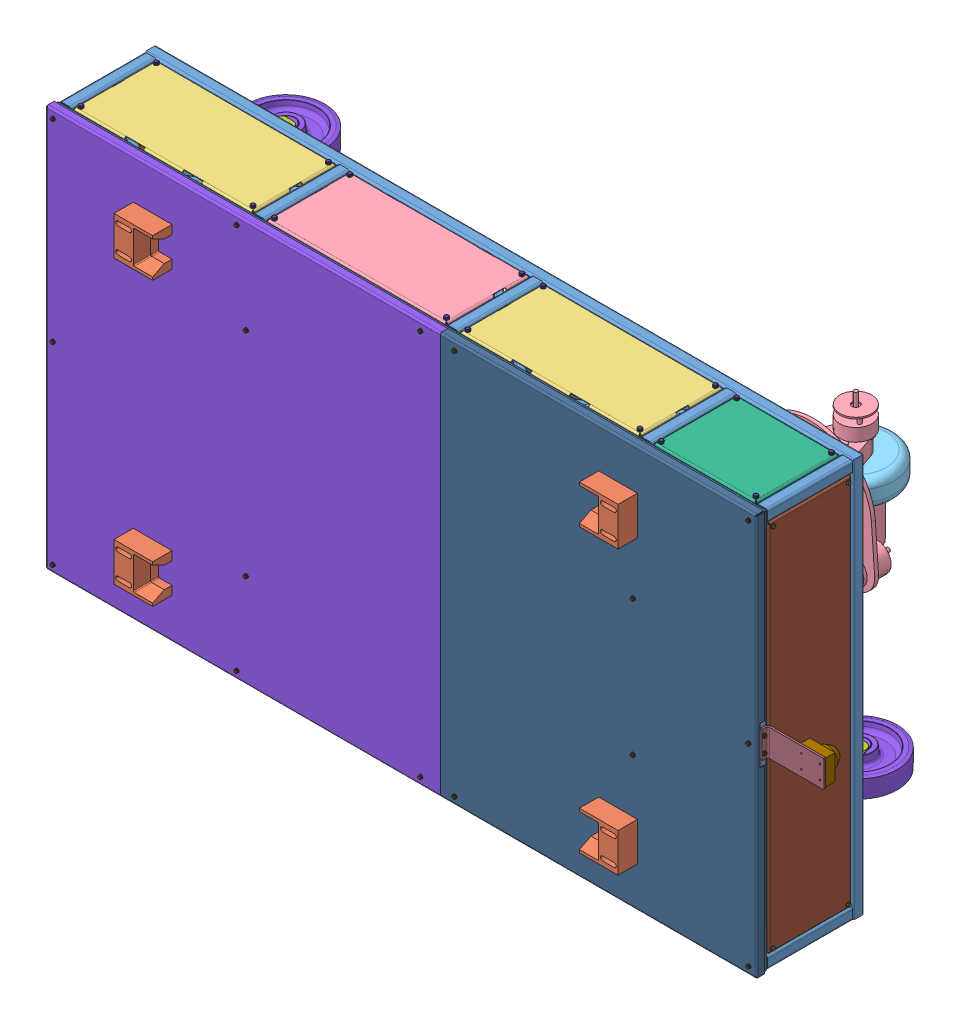
SolidWorks assembly spartaco_bot_V1, configuration Default. Lengths in mm.
Overall size (1986.1 1042.2 588.68).
206 component instances, 48 part files, 26 mates.
Components (placement in the parent):
- robot_body-1: robot_body [Default] at (-881.7629 -500.0018 -180.7451) x (0 -1 0) z (-1 0 0) size (1042.2 351.5 1986.1)
  - 00-A-PT0046 (1).step-1: 00-A-PT0046 (1).step [Default] at origin size (1042.2 306.3 1986.1)
    - 00-P-PT0151_Default_A macchina_.step-1: 00-P-PT0151_Default_A macchina_.step [Default] at origin size (1030 285 1830)
    - 00-P-PT0177.step-1: 00-P-PT0177.step [Default] at (-500 125 15) size (965 215 15)
    - 00-P-PT0153.step-1: 00-P-PT0153.step [Default] at (-1015 125 -250) x (0 0 1) z (-1 0 0) size (465 215 15)
    - 00-P-PT0153.step-2: 00-P-PT0153.step [Default] at (15 125 -250) x (0 0 -1) z (1 0 0) size (465 215 15)
    - 00-P-PT0153.step-3: 00-P-PT0153.step [Default] at (15 125 -1250) x (0 0 -1) z (1 0 0) size (465 215 15)
    - 00-P-PT0153.step-4: 00-P-PT0153.step [Default] at (-1015 125 -1250) x (0 0 1) z (-1 0 0) size (465 215 15)
    - 00-P-PT0169.step-1: 00-P-PT0169.step [Default] at (-1015 125 -750) x (0 0 1) z (-1 0 0) size (465 215 15)
    - 00-P-PT0154.step-1: 00-P-PT0154.step [Default] at (-500 -35 -750) x (0 0 1) z (-1 0 0) size (525 53 557)
    - 00-P-PT0168.step-1: 00-P-PT0168.step [Default] at (15 125 -1650) x (0 0 -1) z (1 0 0) size (265 215 15)
    - 00-P-PT0168.step-2: 00-P-PT0168.step [Default] at (-1015 125 -1650) x (0 0 1) z (-1 0 0) size (265 215 15)
    - 00-A-PT0167.step-1: 00-A-PT0167.step [Default] at (-500 -31 -590) size (500 35 45)
    - 00-P-PT0169.step-2: 00-P-PT0169.step [Default] at (15 125 -750) x (0 0 -1) z (1 0 0) size (465 215 15)
    - 00-A-PT0167.step-2: 00-A-PT0167.step [Default] at (-500 -31 -910) x (-1 0 0) z (0 0 -1) size (500 35 45)
    - 00-P-PT0174.step-1: 00-P-PT0174.step [Default] at (-500 266.5 -899.5) x (0 0 1) z (-1 0 0) size (1020 20 1038.01)
    - 00-P-PT0173.step-1: 00-P-PT0173.step [Default] at (-25 15 -990) x (0 0 1) z (1 0 0) size (500 2 950)
    - 00-P-PT0171.step-1: 00-P-PT0171.step [Default] at (-500 266.5 -899.5) x (0 0 -1) z (1 0 0) size (818 20 1038.01)
    - 00-p-pt0152.step-1: 00-p-pt0152.step [Default] at (-500 125 -1815) x (-1 0 0) z (0 0 -1) size (965 215 15)
    - 00-P-PT0175.step-1: 00-P-PT0175.step [Default] at (-25 17 -505) x (0 0 -1) z (1 0 0) size (190 2 950)
    - 00-p-pt0176.step-1: 00-p-pt0176.step [Default] at (-535 234.8 -1815) size (70 20 150)
    - Rosetta Piana UNI6592_130909006.step-1: Rosetta Piana UNI6592_130909006.step [Default] at (-1015.8 27.5 -1527.5) x (0 -1 0) z (0 0 1) size (11 1.6 11)
    - Rosetta Piana UNI6592_130909006.step-2: Rosetta Piana UNI6592_130909006.step [Default] at (-1015.8 222.5 -1527.5) x (0 -1 0) z (0 0 1) size (11 1.6 11)
    - Rosetta Piana UNI6592_130909006.step-3: Rosetta Piana UNI6592_130909006.step [Default] at (-1015.8 222.5 -1772.5) x (0 -1 0) z (0 0 1) size (11 1.6 11)
    - Rosetta Piana UNI6592_130909006.step-4: Rosetta Piana UNI6592_130909006.step [Default] at (-1015.8 27.5 -1772.5) x (0 -1 0) z (0 0 1) size (11 1.6 11)
    - Rosetta Piana UNI6592_130909006.step-5: Rosetta Piana UNI6592_130909006.step [Default] at (-1015.8 27.5 -1472.5) x (0 -1 0) z (0 0 1) size (11 1.6 11)
    - Rosetta Piana UNI6592_130909006.step-6: Rosetta Piana UNI6592_130909006.step [Default] at (-1015.8 27.5 -1027.5) x (0 0 -1) z (0 -1 0) size (11 1.6 11)
    - Rosetta Piana UNI6592_130909006.step-7: Rosetta Piana UNI6592_130909006.step [Default] at (-1015.8 222.5 -972.5) x (0 -1 0) z (0 0 1) size (11 1.6 11)
    - Rosetta Piana UNI6592_130909006.step-8: Rosetta Piana UNI6592_130909006.step [Default] at (-1015.8 222.5 -527.5) x (0 -1 0) z (0 0 1) size (11 1.6 11)
    - Rosetta Piana UNI6592_130909006.step-9: Rosetta Piana UNI6592_130909006.step [Default] at (-1015.8 27.5 -472.5) x (0 -1 0) z (0 0 1) size (11 1.6 11)
    - Rosetta Piana UNI6592_130909006.step-10: Rosetta Piana UNI6592_130909006.step [Default] at (-1015.8 27.5 -27.5) x (0 -1 0) z (0 0 1) size (11 1.6 11)
    - Rosetta Piana UNI6592_130909006.step-11: Rosetta Piana UNI6592_130909006.step [Default] at (-972.5 222.5 0.6) x (1 0 0) z (0 1 0) size (11 1.6 11)
    - Rosetta Piana UNI6592_130909006.step-12: Rosetta Piana UNI6592_130909006.step [Default] at (-972.5 27.5 15.8) x (1 0 0) z (0 1 0) size (11 1.6 11)
    - Rosetta Piana UNI6592_130909006.step-13: Rosetta Piana UNI6592_130909006.step [Default] at (-27.5 27.5 15.8) x (1 0 0) z (0 1 0) size (11 1.6 11)
    - Rosetta Piana UNI6592_130909006.step-14: Rosetta Piana UNI6592_130909006.step [Default] at (15.8 27.5 -27.5) x (0 1 0) z (0 0 1) size (11 1.6 11)
    - Rosetta Piana UNI6592_130909006.step-15: Rosetta Piana UNI6592_130909006.step [Default] at (15.8 27.5 -472.5) x (0 1 0) z (0 0 1) size (11 1.6 11)
    - Rosetta Piana UNI6592_130909006.step-16: Rosetta Piana UNI6592_130909006.step [Default] at (15.8 222.5 -527.5) x (0 1 0) z (0 0 1) size (11 1.6 11)
    - Rosetta Piana UNI6592_130909006.step-17: Rosetta Piana UNI6592_130909006.step [Default] at (15.8 222.5 -972.5) x (0 1 0) z (0 0 1) size (11 1.6 11)
    - Rosetta Piana UNI6592_130909006.step-18: Rosetta Piana UNI6592_130909006.step [Default] at (15.8 27.5 -1027.5) x (0 1 0) z (0 0 1) size (11 1.6 11)
    - Rosetta Piana UNI6592_130909006.step-19: Rosetta Piana UNI6592_130909006.step [Default] at (15.8 27.5 -1472.5) x (0 1 0) z (0 0 1) size (11 1.6 11)
    - Rosetta Piana UNI6592_130909006.step-20: Rosetta Piana UNI6592_130909006.step [Default] at (15.8 27.5 -1527.5) x (0 1 0) z (0 0 1) size (11 1.6 11)
    - Rosetta Piana UNI6592_130909006.step-21: Rosetta Piana UNI6592_130909006.step [Default] at (15.8 27.5 -1772.5) x (0 1 0) z (0 0 1) size (11 1.6 11)
    - Rosetta Piana UNI6592_130909006.step-22: Rosetta Piana UNI6592_130909006.step [Default] at (15.8 222.5 -1527.5) x (0 1 0) z (0 0 1) size (11 1.6 11)
    - Rosetta Piana UNI6592_130909006.step-23: Rosetta Piana UNI6592_130909006.step [Default] at (15.8 222.5 -1772.5) x (0 1 0) z (0 0 1) size (11 1.6 11)
    - Rosetta Piana UNI6592_130909005.step-1: Rosetta Piana UNI6592_130909005.step [Default] at (-27.5 27.5 -1815.4) x (1 0 0) z (0 -1 0) size (10 0.8 10)
    - Rosetta Piana UNI6592_130909005.step-2: Rosetta Piana UNI6592_130909005.step [Default] at (-27.5 222.5 -1815.4) x (1 0 0) z (0 -1 0) size (10 0.8 10)
    - Rosetta Piana UNI6592_130909005.step-3: Rosetta Piana UNI6592_130909005.step [Default] at (-972.5 27.5 -1815.4) x (1 0 0) z (0 -1 0) size (10 0.8 10)
    - Rosetta Piana UNI6592_130909005.step-4: Rosetta Piana UNI6592_130909005.step [Default] at (-972.5 222.5 -1815.4) x (1 0 0) z (0 -1 0) size (10 0.8 10)
    - Rosetta Piana UNI6592_130909005.step-5: Rosetta Piana UNI6592_130909005.step [Default] at (-750 18.4 -500) x (0.837169 0 0.546944) z (0.546944 0 -0.837169) size (10 0.8 10)
    - Rosetta Piana UNI6592_130909005.step-6: Rosetta Piana UNI6592_130909005.step [Default] at (-500 18.4 -500) x (0.837169 0 0.546944) z (0.546944 0 -0.837169) size (10 0.8 10)
    - Rosetta Piana UNI6592_130909005.step-7: Rosetta Piana UNI6592_130909005.step [Default] at (-250 18.4 -500) x (0.837169 0 0.546944) z (0.546944 0 -0.837169) size (10 0.8 10)
    - Rosetta Piana UNI6592_130909005.step-8: Rosetta Piana UNI6592_130909005.step [Default] at (-250 18.4 -1000) x (0.837169 0 0.546944) z (0.546944 0 -0.837169) size (10 0.8 10)
    - Rosetta Piana UNI6592_130909005.step-9: Rosetta Piana UNI6592_130909005.step [Default] at (-500 18.4 -1000) x (0.837169 0 0.546944) z (0.546944 0 -0.837169) size (10 0.8 10)
    - Rosetta Piana UNI6592_130909005.step-10: Rosetta Piana UNI6592_130909005.step [Default] at (-750 18.4 -1000) x (0.837169 0 0.546944) z (0.546944 0 -0.837169) size (10 0.8 10)
    - V.T.E. Zinc UNI 5739_130328056.step-1: V.T.E. Zinc UNI 5739_130328056.step [Default] at (-750 19.3 -500) size (9.24 24 9.25)
    - V.T.E. Zinc UNI 5739_130328056.step-2: V.T.E. Zinc UNI 5739_130328056.step [Default] at (-500 19.3 -500) size (9.24 24 9.25)
    - V.T.E. Zinc UNI 5739_130328056.step-3: V.T.E. Zinc UNI 5739_130328056.step [Default] at (-250 19.3 -500) size (9.24 24 9.25)
    - V.T.E. Zinc UNI 5739_130328056.step-4: V.T.E. Zinc UNI 5739_130328056.step [Default] at (-250 19.3 -1000) size (9.24 24 9.25)
    - V.T.E. Zinc UNI 5739_130328056.step-5: V.T.E. Zinc UNI 5739_130328056.step [Default] at (-500 19.3 -1000) size (9.24 24 9.25)
    - V.T.E. Zinc UNI 5739_130328056.step-6: V.T.E. Zinc UNI 5739_130328056.step [Default] at (-750 19.3 -1000) size (9.24 24 9.25)
    - Rosetta Piana UNI6592_130909006.step-24: Rosetta Piana UNI6592_130909006.step [Default] at (15.8 222.5 -27.5) x (0 1 0) z (0 0 1) size (11 1.6 11)
    - Rosetta Piana UNI6592_130909006.step-25: Rosetta Piana UNI6592_130909006.step [Default] at (15.8 222.5 -472.5) x (0 1 0) z (0 0 1) size (11 1.6 11)
    - Rosetta Piana UNI6592_130909006.step-26: Rosetta Piana UNI6592_130909006.step [Default] at (15.8 27.5 -527.5) x (0 1 0) z (0 0 1) size (11 1.6 11)
    - Rosetta Piana UNI6592_130909006.step-27: Rosetta Piana UNI6592_130909006.step [Default] at (15.8 27.5 -972.5) x (0 1 0) z (0 0 1) size (11 1.6 11)
    - Rosetta Piana UNI6592_130909006.step-28: Rosetta Piana UNI6592_130909006.step [Default] at (15.8 222.5 -1027.5) x (0 1 0) z (0 0 1) size (11 1.6 11)
    - Rosetta Piana UNI6592_130909006.step-29: Rosetta Piana UNI6592_130909006.step [Default] at (15.8 222.5 -1472.5) x (0 1 0) z (0 0 1) size (11 1.6 11)
    - Rosetta Piana UNI6592_130909006.step-30: Rosetta Piana UNI6592_130909006.step [Default] at (-1015.8 222.5 -1472.5) x (0 -1 0) z (0 0 1) size (11 1.6 11)
    - Rosetta Piana UNI6592_130909006.step-31: Rosetta Piana UNI6592_130909006.step [Default] at (-1015.8 222.5 -1027.5) x (0 -1 0) z (0 0 1) size (11 1.6 11)
    - Rosetta Piana UNI6592_130909006.step-32: Rosetta Piana UNI6592_130909006.step [Default] at (-1015.8 27.5 -972.5) x (0 -1 0) z (0 0 1) size (11 1.6 11)
    - Rosetta Piana UNI6592_130909006.step-33: Rosetta Piana UNI6592_130909006.step [Default] at (-1015.8 27.5 -527.5) x (0 -1 0) z (0 0 1) size (11 1.6 11)
    - Rosetta Piana UNI6592_130909006.step-34: Rosetta Piana UNI6592_130909006.step [Default] at (-1015.8 222.5 -472.5) x (0 -1 0) z (0 0 1) size (11 1.6 11)
    - Rosetta Piana UNI6592_130909006.step-35: Rosetta Piana UNI6592_130909006.step [Default] at (-1015.8 222.5 -27.5) x (0 -1 0) z (0 0 1) size (11 1.6 11)
    - Rosetta Piana UNI6592_130909005.step-11: Rosetta Piana UNI6592_130909005.step [Default] at (-1 266.9 -0.5) x (0.837169 0 0.546944) z (0.546944 0 -0.837169) size (10 0.8 10)
    - Rosetta Piana UNI6592_130909005.step-12: Rosetta Piana UNI6592_130909005.step [Default] at (-1 266.9 -475.5) x (0.837169 0 0.546944) z (0.546944 0 -0.837169) size (10 0.8 10)
    - Rosetta Piana UNI6592_130909005.step-13: Rosetta Piana UNI6592_130909005.step [Default] at (-500 266.9 -0.5) x (0.837169 0 0.546944) z (0.546944 0 -0.837169) size (10 0.8 10)
    - Rosetta Piana UNI6592_130909005.step-14: Rosetta Piana UNI6592_130909005.step [Default] at (-225 266.9 -499.5) x (0.837169 0 0.546944) z (0.546944 0 -0.837169) size (10 0.8 10)
    - Rosetta Piana UNI6592_130909005.step-15: Rosetta Piana UNI6592_130909005.step [Default] at (-775 266.9 -499.5) x (0.837169 0 0.546944) z (0.546944 0 -0.837169) size (10 0.8 10)
    - Rosetta Piana UNI6592_130909005.step-16: Rosetta Piana UNI6592_130909005.step [Default] at (-999 266.9 -475.5) x (0.837169 0 0.546944) z (0.546944 0 -0.837169) size (10 0.8 10)
    - Rosetta Piana UNI6592_130909005.step-17: Rosetta Piana UNI6592_130909005.step [Default] at (-999 266.9 -0.5) x (0.837169 0 0.546944) z (0.546944 0 -0.837169) size (10 0.8 10)
    - Rosetta Piana UNI6592_130909005.step-18: Rosetta Piana UNI6592_130909005.step [Default] at (-1 266.9 -950.5) x (0.837169 0 0.546944) z (0.546944 0 -0.837169) size (10 0.8 10)
    - Rosetta Piana UNI6592_130909005.step-19: Rosetta Piana UNI6592_130909005.step [Default] at (-1 266.9 -1038.5) x (0.837169 0 0.546944) z (0.546944 0 -0.837169) size (10 0.8 10)
    - Rosetta Piana UNI6592_130909005.step-20: Rosetta Piana UNI6592_130909005.step [Default] at (-325 266.9 -1500) x (0.837169 0 0.546944) z (0.546944 0 -0.837169) size (10 0.8 10)
    - Rosetta Piana UNI6592_130909005.step-21: Rosetta Piana UNI6592_130909005.step [Default] at (-1 266.9 -1798.5) x (0.837169 0 0.546944) z (0.546944 0 -0.837169) size (10 0.8 10)
    - Rosetta Piana UNI6592_130909005.step-22: Rosetta Piana UNI6592_130909005.step [Default] at (-500 266.9 -1798.5) x (0.837169 0 0.546944) z (0.546944 0 -0.837169) size (10 0.8 10)
    - Rosetta Piana UNI6592_130909005.step-23: Rosetta Piana UNI6592_130909005.step [Default] at (-675 266.9 -1500) x (0.837169 0 0.546944) z (0.546944 0 -0.837169) size (10 0.8 10)
    - Rosetta Piana UNI6592_130909005.step-24: Rosetta Piana UNI6592_130909005.step [Default] at (-999 266.9 -1798.5) x (0.837169 0 0.546944) z (0.546944 0 -0.837169) size (10 0.8 10)
    - Rosetta Piana UNI6592_130909005.step-25: Rosetta Piana UNI6592_130909005.step [Default] at (-999 266.9 -1038.5) x (0.837169 0 0.546944) z (0.546944 0 -0.837169) size (10 0.8 10)
    - Rosetta Piana UNI6592_130909005.step-26: Rosetta Piana UNI6592_130909005.step [Default] at (-999 266.9 -950.5) x (0.837169 0 0.546944) z (0.546944 0 -0.837169) size (10 0.8 10)
    - Rosetta Piana UNI6592_130909005.step-27: Rosetta Piana UNI6592_130909005.step [Default] at (-480 249.8 -1820.4) x (1 0 0) z (0 -1 0) size (10 0.8 10)
    - Rosetta Piana UNI6592_130909005.step-28: Rosetta Piana UNI6592_130909005.step [Default] at (-520 249.8 -1820.4) x (1 0 0) z (0 -1 0) size (10 0.8 10)
    - V.T.E. Zinc UNI 5739_130328089.step-1: V.T.E. Zinc UNI 5739_130328089.step [Default] at (-1017.1 222.5 -1772.5) x (0 1 0) z (0 0 1) size (11.56 34.5 11.57)
    - V.T.E. Zinc UNI 5739_130328089.step-2: V.T.E. Zinc UNI 5739_130328089.step [Default] at (-1017.1 222.5 -1527.5) x (0 1 0) z (0 0 1) size (11.56 34.5 11.57)
    - V.T.E. Zinc UNI 5739_130328089.step-3: V.T.E. Zinc UNI 5739_130328089.step [Default] at (-1017.1 27.5 -1772.5) x (0 1 0) z (0 0 1) size (11.56 34.5 11.57)
    - V.T.E. Zinc UNI 5739_130328089.step-4: V.T.E. Zinc UNI 5739_130328089.step [Default] at (-1017.1 27.5 -1527.5) x (0 1 0) z (0 0 1) size (11.56 34.5 11.57)
    - V.T.E. Zinc UNI 5739_130328089.step-5: V.T.E. Zinc UNI 5739_130328089.step [Default] at (-1017.1 27.5 -1472.5) x (0 1 0) z (0 0 1) size (11.56 34.5 11.57)
    - V.T.E. Zinc UNI 5739_130328089.step-6: V.T.E. Zinc UNI 5739_130328089.step [Default] at (-1017.1 27.5 -1027.5) x (0 1 0) z (0 0 1) size (11.56 34.5 11.57)
    - V.T.E. Zinc UNI 5739_130328089.step-7: V.T.E. Zinc UNI 5739_130328089.step [Default] at (-1017.1 222.5 -972.5) x (0 1 0) z (0 0 1) size (11.56 34.5 11.57)
    - V.T.E. Zinc UNI 5739_130328089.step-8: V.T.E. Zinc UNI 5739_130328089.step [Default] at (-1017.1 222.5 -527.5) x (0 1 0) z (0 0 1) size (11.56 34.5 11.57)
    - V.T.E. Zinc UNI 5739_130328089.step-9: V.T.E. Zinc UNI 5739_130328089.step [Default] at (-1017.1 27.5 -472.5) x (0 1 0) z (0 0 1) size (11.56 34.5 11.57)
    - V.T.E. Zinc UNI 5739_130328089.step-10: V.T.E. Zinc UNI 5739_130328089.step [Default] at (-1017.1 27.5 -27.5) x (0 1 0) z (0 0 1) size (11.56 34.5 11.57)
    - V.T.E. Zinc UNI 5739_130328089.step-11: V.T.E. Zinc UNI 5739_130328089.step [Default] at (-972.5 27.5 17.1) x (1 0 0) z (0 -1 0) size (11.56 34.5 11.57)
    - V.T.E. Zinc UNI 5739_130328089.step-12: V.T.E. Zinc UNI 5739_130328089.step [Default] at (-27.5 27.5 17.1) x (1 0 0) z (0 -1 0) size (11.56 34.5 11.57)
    - V.T.E. Zinc UNI 5739_130328089.step-13: V.T.E. Zinc UNI 5739_130328089.step [Default] at (17.1 27.5 -27.5) x (0 -1 0) z (0 0 1) size (11.56 34.5 11.57)
    - V.T.E. Zinc UNI 5739_130328089.step-14: V.T.E. Zinc UNI 5739_130328089.step [Default] at (17.1 27.5 -472.5) x (0 -1 0) z (0 0 1) size (11.56 34.5 11.57)
    - V.T.E. Zinc UNI 5739_130328089.step-15: V.T.E. Zinc UNI 5739_130328089.step [Default] at (17.1 222.5 -527.5) x (0 -1 0) z (0 0 1) size (11.56 34.5 11.57)
    - V.T.E. Zinc UNI 5739_130328089.step-16: V.T.E. Zinc UNI 5739_130328089.step [Default] at (17.1 222.5 -972.5) x (0 -1 0) z (0 0 1) size (11.56 34.5 11.57)
    - V.T.E. Zinc UNI 5739_130328089.step-17: V.T.E. Zinc UNI 5739_130328089.step [Default] at (17.1 27.5 -1027.5) x (0 -1 0) z (0 0 1) size (11.56 34.5 11.57)
    - V.T.E. Zinc UNI 5739_130328089.step-18: V.T.E. Zinc UNI 5739_130328089.step [Default] at (17.1 27.5 -1472.5) x (0 -1 0) z (0 0 1) size (11.56 34.5 11.57)
    - V.T.E. Zinc UNI 5739_130328089.step-19: V.T.E. Zinc UNI 5739_130328089.step [Default] at (17.1 27.5 -1527.5) x (0 -1 0) z (0 0 1) size (11.56 34.5 11.57)
    - V.T.E. Zinc UNI 5739_130328089.step-20: V.T.E. Zinc UNI 5739_130328089.step [Default] at (17.1 27.5 -1772.5) x (0 -1 0) z (0 0 1) size (11.56 34.5 11.57)
    - V.T.E. Zinc UNI 5739_130328089.step-21: V.T.E. Zinc UNI 5739_130328089.step [Default] at (17.1 222.5 -1527.5) x (0 -1 0) z (0 0 1) size (11.56 34.5 11.57)
    - V.T.E. Zinc UNI 5739_130328089.step-22: V.T.E. Zinc UNI 5739_130328089.step [Default] at (17.1 222.5 -1772.5) x (0 -1 0) z (0 0 1) size (11.56 34.5 11.57)
    - Rosetta Piana UNI6592_130909006.step-36: Rosetta Piana UNI6592_130909006.step [Default] at (-972.5 222.5 15.8) x (1 0 0) z (0 1 0) size (11 1.6 11)
    - Rosetta Piana UNI6592_130909006.step-37: Rosetta Piana UNI6592_130909006.step [Default] at (-27.5 222.5 15.8) x (1 0 0) z (0 1 0) size (11 1.6 11)
    - V.T.E. Zinc UNI 5739_130328089.step-23: V.T.E. Zinc UNI 5739_130328089.step [Default] at (-27.5 222.5 17.1) x (1 0 0) z (0 -1 0) size (11.56 34.5 11.57)
    - V.T.E. Zinc UNI 5739_130328089.step-24: V.T.E. Zinc UNI 5739_130328089.step [Default] at (-972.5 222.5 17.1) x (1 0 0) z (0 -1 0) size (11.56 34.5 11.57)
    - V.T.E. Zinc UNI 5739_130328056.step-7: V.T.E. Zinc UNI 5739_130328056.step [Default] at (-27.5 27.5 -1816.3) x (0.960124 0.279576 0) z (-0.279576 0.960124 0) size (9.24 24 9.25)
    - V.T.E. Zinc UNI 5739_130328056.step-8: V.T.E. Zinc UNI 5739_130328056.step [Default] at (-27.5 222.5 -1816.3) x (-0.948121 0.317909 0) z (-0.317909 -0.948121 0) size (9.24 24 9.25)
    - V.T.E. Zinc UNI 5739_130328056.step-9: V.T.E. Zinc UNI 5739_130328056.step [Default] at (-972.5 27.5 -1816.3) x (1 0 0) z (0 1 0) size (9.24 24 9.25)
    - V.T.E. Zinc UNI 5739_130328056.step-10: V.T.E. Zinc UNI 5739_130328056.step [Default] at (-972.5 222.5 -1816.3) x (1 0 0) z (0 1 0) size (9.24 24 9.25)
    - V.T.E. Zinc UNI 5739_130328089.step-25: V.T.E. Zinc UNI 5739_130328089.step [Default] at (17.1 222.5 -27.5) x (0 -1 0) z (0 0 1) size (11.56 34.5 11.57)
    - V.T.E. Zinc UNI 5739_130328089.step-26: V.T.E. Zinc UNI 5739_130328089.step [Default] at (17.1 222.5 -472.5) x (0 -1 0) z (0 0 1) size (11.56 34.5 11.57)
    - V.T.E. Zinc UNI 5739_130328089.step-27: V.T.E. Zinc UNI 5739_130328089.step [Default] at (17.1 27.5 -527.5) x (0 -1 0) z (0 0 1) size (11.56 34.5 11.57)
    - V.T.E. Zinc UNI 5739_130328089.step-28: V.T.E. Zinc UNI 5739_130328089.step [Default] at (17.1 27.5 -972.5) x (0 -1 0) z (0 0 1) size (11.56 34.5 11.57)
    - V.T.E. Zinc UNI 5739_130328089.step-29: V.T.E. Zinc UNI 5739_130328089.step [Default] at (17.1 222.5 -1027.5) x (0 -1 0) z (0 0 1) size (11.56 34.5 11.57)
    - V.T.E. Zinc UNI 5739_130328089.step-30: V.T.E. Zinc UNI 5739_130328089.step [Default] at (17.1 222.5 -1472.5) x (0 -1 0) z (0 0 1) size (11.56 34.5 11.57)
    - V.T.E. Zinc UNI 5739_130328089.step-31: V.T.E. Zinc UNI 5739_130328089.step [Default] at (-1017.1 222.5 -1472.5) x (0 1 0) z (0 0 1) size (11.56 34.5 11.57)
    - V.T.E. Zinc UNI 5739_130328089.step-32: V.T.E. Zinc UNI 5739_130328089.step [Default] at (-1017.1 222.5 -1027.5) x (0 1 0) z (0 0 1) size (11.56 34.5 11.57)
    - V.T.E. Zinc UNI 5739_130328089.step-33: V.T.E. Zinc UNI 5739_130328089.step [Default] at (-1017.1 27.5 -527.5) x (0 1 0) z (0 0 1) size (11.56 34.5 11.57)
    - V.T.E. Zinc UNI 5739_130328089.step-34: V.T.E. Zinc UNI 5739_130328089.step [Default] at (-1017.1 222.5 -472.5) x (0 1 0) z (0 0 1) size (11.56 34.5 11.57)
    - V.T.E. Zinc UNI 5739_130328089.step-35: V.T.E. Zinc UNI 5739_130328089.step [Default] at (-1017.1 222.5 -27.5) x (0 1 0) z (0 0 1) size (11.56 34.5 11.57)
    - V.T.E. Zinc UNI 5739_130328089.step-36: V.T.E. Zinc UNI 5739_130328089.step [Default] at (-1017.1 27.5 -972.5) x (0 1 0) z (0 0 1) size (11.56 34.5 11.57)
    - V.T.E. Zinc UNI 5739 M5_Vite TE M5X16.step-1: V.T.E. Zinc UNI 5739 M5_Vite TE M5X16.step [Default] at (-1 267.8 -0.5) size (9.24 20 9.25)
    - V.T.E. Zinc UNI 5739 M5_Vite TE M5X16.step-2: V.T.E. Zinc UNI 5739 M5_Vite TE M5X16.step [Default] at (-500 267.8 -0.5) size (9.24 20 9.25)
    - V.T.E. Zinc UNI 5739 M5_Vite TE M5X16.step-3: V.T.E. Zinc UNI 5739 M5_Vite TE M5X16.step [Default] at (-225 267.8 -499.5) size (9.24 20 9.25)
    - V.T.E. Zinc UNI 5739 M5_Vite TE M5X16.step-4: V.T.E. Zinc UNI 5739 M5_Vite TE M5X16.step [Default] at (-1 267.8 -475.5) size (9.24 20 9.25)
    - V.T.E. Zinc UNI 5739 M5_Vite TE M5X16.step-5: V.T.E. Zinc UNI 5739 M5_Vite TE M5X16.step [Default] at (-1 267.8 -950.5) size (9.24 20 9.25)
    - V.T.E. Zinc UNI 5739 M5_Vite TE M5X16.step-6: V.T.E. Zinc UNI 5739 M5_Vite TE M5X16.step [Default] at (-1 267.8 -1038.5) size (9.24 20 9.25)
    - V.T.E. Zinc UNI 5739 M5_Vite TE M5X16.step-7: V.T.E. Zinc UNI 5739 M5_Vite TE M5X16.step [Default] at (-1 267.8 -1798.5) size (9.24 20 9.25)
    - V.T.E. Zinc UNI 5739 M5_Vite TE M5X16.step-8: V.T.E. Zinc UNI 5739 M5_Vite TE M5X16.step [Default] at (-325 267.8 -1500) size (9.24 20 9.25)
    - V.T.E. Zinc UNI 5739 M5_Vite TE M5X16.step-9: V.T.E. Zinc UNI 5739 M5_Vite TE M5X16.step [Default] at (-500 267.8 -1798.5) size (9.24 20 9.25)
    - V.T.E. Zinc UNI 5739 M5_Vite TE M5X16.step-10: V.T.E. Zinc UNI 5739 M5_Vite TE M5X16.step [Default] at (-675 267.8 -1500) size (9.24 20 9.25)
    - V.T.E. Zinc UNI 5739 M5_Vite TE M5X16.step-11: V.T.E. Zinc UNI 5739 M5_Vite TE M5X16.step [Default] at (-999 267.8 -1798.5) size (9.24 20 9.25)
    - V.T.E. Zinc UNI 5739 M5_Vite TE M5X16.step-12: V.T.E. Zinc UNI 5739 M5_Vite TE M5X16.step [Default] at (-999 267.8 -1038.5) size (9.24 20 9.25)
    - V.T.E. Zinc UNI 5739 M5_Vite TE M5X16.step-13: V.T.E. Zinc UNI 5739 M5_Vite TE M5X16.step [Default] at (-999 267.8 -950.5) size (9.24 20 9.25)
    - V.T.E. Zinc UNI 5739 M5_Vite TE M5X16.step-14: V.T.E. Zinc UNI 5739 M5_Vite TE M5X16.step [Default] at (-999 267.8 -0.5) size (9.24 20 9.25)
    - V.T.E. Zinc UNI 5739 M5_Vite TE M5X16.step-15: V.T.E. Zinc UNI 5739 M5_Vite TE M5X16.step [Default] at (-480 249.8 -1821.3) x (1 0 0) z (0 1 0) size (9.24 20 9.25)
    - V.T.E. Zinc UNI 5739 M5_Vite TE M5X16.step-16: V.T.E. Zinc UNI 5739 M5_Vite TE M5X16.step [Default] at (-520 249.8 -1821.3) x (1 0 0) z (0 1 0) size (9.24 20 9.25)
    - V.T.E. Zinc UNI 5739 M5_Vite TE M5X16.step-17: V.T.E. Zinc UNI 5739 M5_Vite TE M5X16.step [Default] at (-999 267.8 -475.5) size (9.24 20 9.25)
    - V.T.E. Zinc UNI 5739 M5_Vite TE M5X16.step-18: V.T.E. Zinc UNI 5739 M5_Vite TE M5X16.step [Default] at (-775 267.8 -499.5) size (9.24 20 9.25)
    - 00-P-PT0178.step-1: 00-P-PT0178.step [Default] at (-500 17 -1015) x (0 0 -1) z (1 0 0) size (50 240 600)
  - cuneo_pedana-1: cuneo_pedana [Default] at (-865 266.5 -207) size (100 50 100)
  - cuneo_pedana-2: cuneo_pedana [Default] at (-135 266.5 -1510) x (-1 0 0) z (0 0 -1) size (100 50 100)
  - cuneo_pedana-3: cuneo_pedana [Default] at (-865 266.5 -1510) x (-1 0 0) z (0 0 -1) size (100 50 100)
  - cuneo_pedana-4: cuneo_pedana [Default] at (-135 266.5 -207) size (100 50 100)
- batteria-1: batteria [Default] at (-131.7629 -0.0018 -212.7451) x (0 -1 0) z (-1 0 0) size (569 275 320)
- MRT05-1: MRT05 [Default] at (-737.9796 -364.3122 -288.3365) x (-1 0 0) z (0 1 0) size (337.24 246.99 360.81)
  - MRT05-1: MRT05 [Default] at (-16.2167 -3.4086 117.2864) x (-1 0 0) z (0 0 -1) size (337.24 211.1 360.81)
  - MRT05_wheel-1: MRT05_wheel [Default] at (-16.2167 -60.4032 39.3104) x (0 0 1) z (-1 0 0) size (71 198 198)
- MRT05-2: MRT05 [Default] at (742.0204 285.6878 -288.3365) x (-1 0 0) z (0 1 0) size (337.24 246.99 360.81)
  - MRT05-1: MRT05 [Default] at (-16.2167 -3.4086 117.2864) x (-1 0 0) z (0 0 -1) size (337.24 211.1 360.81)
  - MRT05_wheel-1: MRT05_wheel [Default] at (-16.2167 -60.4032 39.3104) x (0 0 1) z (-1 0 0) size (71 198 198)
- castor_pivot-1: castor_pivot [Default] at (823.2371 -325.0018 -210.5605) x (1 0 0) z (0 0 -1) size (204.58 110 156.49)
  - piastra_pivot-1: piastra_pivot [Default] at (0 0 -9.8154) size (135 110 24.79)
  - pivot-1: pivot [Default] at (-57.8 -35.5 138.1746) x (1 0 0) z (0 1 0) size (183.58 152.49 93)
- castor_pivot-2: castor_pivot [Default] at (-656.7629 324.9982 -210.5605) x (1 0 0) z (0 0 -1) size (204.58 110 156.49)
  - piastra_pivot-1: piastra_pivot [Default] at (0 0 -9.8154) size (135 110 24.79)
  - pivot-1: pivot [Default] at (-57.8 -35.5 138.1746) x (1 0 0) z (0 1 0) size (183.58 152.49 93)
- wheel_200-1: wheel_200 [Default] at (-714.5629 324.9982 -348.7351) x (0 1 0) z (1 0 0) size (62.5 200 200)
- wheel_200-2: wheel_200 [Default] at (765.4371 -325.0018 -348.7351) x (0 1 0) z (0.999085 0 0.042769) size (62.5 200 200)
- lidar-1: lidar [Default] at (1049.2371 -0.0018 54.0549) x (-1 0 0) z (0 0 -1) size (73 65 60)
- quadro_elettrico_full-1: quadro_elettrico_full [Default] at (403.2371 -0.0018 -163.7451) x (0 1 0) z (0 0 1) size (930 400 160)
  - quadro_elettrico-1: quadro_elettrico [Default] at origin size (930 400 160)
  - minitraction_power_mockup-1: minitraction_power_mockup [Default] at (67.5 -105 10) size (85 130 40)
  - SD-100C-12-1: SD-100C-12 [Default] at (-124.5 -91.125 11.5) x (1 0 0) z (0 -1 0) size (199.09 37.75 98.27)
    - SD-100C-12.stp-1: SD-100C-12.stp [Default] at origin size (199.09 37.75 98.27)
      - SD-100-20201028.stp.stp-1: SD-100-20201028.stp.stp [Default] at origin size (199.09 37.75 98.27)
        - SD-100_STP.ASM.stp-1: SD-100_STP.ASM.stp [Default] at origin size (199.09 37.75 98.27)
          - SD-100_1_ASM.ASM.stp-1: SD-100_1_ASM.ASM.stp [Default] at origin size (199 37.75 98.27)
            - 902-D-80_ASM.ASM.stp-1: 902-D-80_ASM.ASM.stp [Default] at origin size (199 37.75 97.75)
              - 902-D-119_PRT.PRT.stp-1: 902-D-119_PRT.PRT.stp [Default] at origin size (199 37.75 97.75)
              - NUT_PRT.PRT.stp-1: NUT_PRT.PRT.stp [Default] at (-111.528 -1.5 -40.7894) x (-1 0 0) z (0 1 0) size (8 6.93 6)
            - 902-T_PRT.PRT.stp-1: 902-T_PRT.PRT.stp [Default] at (96.5 36.1 -49.375) x (-1 0 0) z (0 0 -1) size (195.5 36.02 96.52)
            - MYLAR_PRT.PRT.stp-1: MYLAR_PRT.PRT.stp [Default] at (79.2081 1.5 46.5396) x (-1 0 0) z (0 -1 0) size (197 95 0.5)
            - HS2_PRT.PRT.stp-1: HS2_PRT.PRT.stp [Default] at (-64.5 -80.2586 -88.3567) x (0 0 1) z (-1 0 0) size (6.4 28 55)
            - PCB_PRT.PRT.stp-1: PCB_PRT.PRT.stp [Default] at (-189.5595 4.5 45.0362) x (1 0 0) z (0 1 0) size (194 95 1.6)
          - T44-BS1R05370120201023_STP.ASM.stp-1: T44-BS1R05370120201023_STP.ASM.stp [Default] at (-82.3888 6.1 -32.875) x (0 0 1) z (0 1 0) size (69.8 18 18.8)
            - 6_PRT.PRT.stp-1: 6_PRT.PRT.stp [Default] at origin size (7.51 7.5 3.96)
            - 2_PRT.PRT.stp-1: 2_PRT.PRT.stp [Default] at origin size (7.5 7.5 3.96)
            - 3_PRT.PRT.stp-1: 3_PRT.PRT.stp [Default] at origin size (7.51 7.5 3.96)
            - 4_PRT.PRT.stp-1: 4_PRT.PRT.stp [Default] at (0 0.8 0) size (69.8 18 18.8)
            - 5_PRT.PRT.stp-1: 5_PRT.PRT.stp [Default] at origin size (7.51 7.5 3.96)
            - 6_PRT_1.PRT.stp-1: 6_PRT_1.PRT.stp [Default] at (9.5 0 0) size (7.51 7.5 3.96)
            - 6_PRT_1_1.PRT.stp-1: 6_PRT_1_1.PRT.stp [Default] at (19 0 0) size (7.51 7.5 3.96)
            - 6_PRT_1_1_1.PRT.stp-1: 6_PRT_1_1_1.PRT.stp [Default] at (28.5 0 0) size (7.51 7.5 3.96)
  - SD-25C-12-1: SD-25C-12 [Default] at (-36.8335 -327.0246 17.8) size (99.05 97.03 36.06)
    - SD-25C-12.stp-1: SD-25C-12.stp [Default] at origin size (99.05 97.03 36.06)
      - RS-50_ASM_15.ASM.stp-1: RS-50_ASM_15.ASM.stp [Default] at origin size (99.05 97.03 36.06)
        - TN1_2.PRT.stp-1: TN1_2.PRT.stp [Default] at (-301.0065 335.8998 37.1723) x (0 0 -1) z (-1 0 0) size (15.25 49.25 14.66)
        - RS-50-CASE-T_21.PRT.stp-1: RS-50-CASE-T_21.PRT.stp [Default] at (0 1.5 1) size (97.05 96.6 36.06)
        - RS-50-CASE-D_28.PRT.stp-1: RS-50-CASE-D_28.PRT.stp [Default] at (-0.5 0.5 0) size (98.5 97 35)
        - RS-50-PCB_2.PRT.stp-1: RS-50-PCB_2.PRT.stp [Default] at (0 -0.6 -0.2033) size (98 95 1.6)
  - minitraction_power_mockup-2: minitraction_power_mockup [Default] at (172.5 -105 10) size (85 130 40)
  - minitraction_power_mockup-3: minitraction_power_mockup [Default] at (277.5 -105 10) size (85 130 40)
  - minitraction_power_mockup-4: minitraction_power_mockup [Default] at (382.5 -105 10) size (85 130 40)
- panda_mockup-1: panda_mockup [Default] at (171.9371 -410.0018 -83.7451) x (0 1 0) z (1 0 0) size (110 160 39.6)
Mates (geometry in assembly coordinates):
- Coincidente2: coincident anti-aligned: plane of robot_body-1/00-A-PT0046 (1).step-1/00-P-PT0154.step-1 through (100.7371 272.4982 -212.7451) normal (0 0 1); plane of batteria-1 through (-131.7629 -0.0018 -212.7451) normal (0 0 -1)
- Larghezza1: width aligned: plane of robot_body-1/00-A-PT0046 (1).step-1/00-P-PT0154.step-1 through (-131.7629 275.4982 -215.7451) normal (0 -1 0); plane of batteria-1 through (-131.7629 -275.5018 -215.7451) normal (0 1 0); plane of robot_body-1/00-A-PT0046 (1).step-1/00-P-PT0154.step-1 through (-291.7629 -270.5018 62.2549) normal (0 -1 0); plane of batteria-1 through (-291.7629 270.4982 62.2549) normal (0 1 0)
- Larghezza2: width anti-aligned: plane of robot_body-1/00-A-PT0046 (1).step-1/00-A-PT0167.step-2 through (28.2371 249.9982 -176.7451) normal (-1 0 0); plane of batteria-1 through (-291.7629 -250.0018 -176.7451) normal (1 0 0); plane of robot_body-1/00-A-PT0046 (1).step-1/00-A-PT0167.step-1 through (28.2371 270.4982 62.2549) normal (1 0 0); plane of batteria-1 through (-291.7629 270.4982 62.2549) normal (-1 0 0)
- Concentrico3: concentric anti-aligned: cylinder of robot_body-1/00-A-PT0046 (1).step-1/00-P-PT0151_Default_A macchina_.step-1 through (-721.7629 -325.0018 -200.7451) axis (0 0 1) radius 5; line of MRT05-1/MRT05-1 through (-721.7629 -325.0018 -155.5154) axis (0 0 -1)
- Coincidente3: coincident anti-aligned: plane of robot_body-1/00-A-PT0046 (1).step-1/00-P-PT0151_Default_A macchina_.step-1 through (-2361.7629 -1150.0018 -200.7451) normal (0 0 -1); plane of MRT05-1/MRT05-1 through (-721.7629 -200.5018 -200.7451) normal (0 0 1)
- Concentrico11: concentric anti-aligned: cylinder of robot_body-1/00-A-PT0046 (1).step-1/00-P-PT0151_Default_A macchina_.step-1 through (758.2371 324.9982 -200.7451) axis (0 0 1) radius 5; line of MRT05-2/MRT05-1 through (758.2371 324.9982 -155.5154) axis (0 0 -1)
- Coincidente6: coincident anti-aligned: plane of robot_body-1/00-A-PT0046 (1).step-1/00-P-PT0151_Default_A macchina_.step-1 through (-881.7629 -500.0018 -200.7451) normal (0 0 -1); plane of MRT05-2/MRT05-1 through (758.2371 449.4982 -200.7451) normal (0 0 1)
- Coincidente7: coincident anti-aligned: plane of robot_body-1/00-A-PT0046 (1).step-1/00-P-PT0151_Default_A macchina_.step-1 through (-881.7629 -1150.0018 -200.7451) normal (0 0 -1); plane of castor_pivot-1/piastra_pivot-1 through (823.2371 -325.0018 -200.7451) normal (0 0 1)
- Concentrico12: concentric aligned: cylinder of robot_body-1/00-A-PT0046 (1).step-1/00-P-PT0151_Default_A macchina_.step-1 through (875.7371 -286.2518 -200.7451) axis (0 0 1) radius 6.5; cylinder of castor_pivot-1/piastra_pivot-1 through (875.7371 -286.2518 -203.7451) axis (0 0 1) radius 5
- Concentrico13: concentric aligned: cylinder of robot_body-1/00-A-PT0046 (1).step-1/00-P-PT0151_Default_A macchina_.step-1 through (875.7371 -363.7518 -200.7451) axis (0 0 1) radius 6.5; cylinder of castor_pivot-1/piastra_pivot-1 through (875.7371 -363.7518 -203.7451) axis (0 0 1) radius 5
- Coincidente8: coincident anti-aligned: plane of robot_body-1/00-A-PT0046 (1).step-1/00-P-PT0151_Default_A macchina_.step-1 through (-2361.7629 -500.0018 -200.7451) normal (0 0 -1); plane of castor_pivot-2/piastra_pivot-1 through (-656.7629 324.9982 -200.7451) normal (0 0 1)
- Concentrico14: concentric aligned: cylinder of robot_body-1/00-A-PT0046 (1).step-1/00-P-PT0151_Default_A macchina_.step-1 through (-604.2629 363.7482 -200.7451) axis (0 0 1) radius 6.5; cylinder of castor_pivot-2/piastra_pivot-1 through (-604.2629 363.7482 -203.7451) axis (0 0 1) radius 5
- Concentrico15: concentric aligned: cylinder of robot_body-1/00-A-PT0046 (1).step-1/00-P-PT0151_Default_A macchina_.step-1 through (-604.2629 286.2482 -200.7451) axis (0 0 1) radius 6.5; cylinder of castor_pivot-2/piastra_pivot-1 through (-604.2629 286.2482 -203.7451) axis (0 0 1) radius 5
- Coincidente11: coincident anti-aligned: plane of robot_body-1/00-A-PT0046 (1).step-1/00-p-pt0176.step-1 through (943.2371 -35.0018 54.0549) normal (0 0 -1); plane of lidar-1 through (1049.2371 -0.0018 54.0549) normal (0 0 1)
- Concentrico16: concentric aligned: cylinder of robot_body-1/00-A-PT0046 (1).step-1/00-p-pt0176.step-1 through (1073.2371 -18.0018 54.0539) axis (0 0 1) radius 2; circle of lidar-1
- Concentrico17: concentric aligned: cylinder of robot_body-1/00-A-PT0046 (1).step-1/00-p-pt0176.step-1 through (1073.2371 17.9982 54.0539) axis (0 0 1) radius 2; cylinder of lidar-1 through (1073.2371 17.9982 49.0549) axis (0 0 1) radius 1.5
- Coincidente12: coincident anti-aligned: plane of robot_body-1/00-A-PT0046 (1).step-1/00-P-PT0173.step-1 through (108.2371 -475.0018 -163.7451) normal (0 0 1); plane of quadro_elettrico_full-1/quadro_elettrico-1 through (403.2371 -0.0018 -163.7451) normal (0 0 -1)
- Larghezza5: width anti-aligned: plane of robot_body-1/00-A-PT0046 (1).step-1/00-P-PT0153.step-4 through (368.2371 513.4982 -55.7451) normal (0 -1 0); plane of quadro_elettrico_full-1/quadro_elettrico-1 through (368.2371 -513.5018 -55.7451) normal (0 1 0); plane of robot_body-1/00-A-PT0046 (1).step-1/00-P-PT0153.step-3 through (203.2371 464.9982 -153.7451) normal (0 1 0); plane of quadro_elettrico_full-1/quadro_elettrico-1 through (203.2371 -465.0018 -153.7451) normal (0 -1 0)
- Coincidente13: coincident anti-aligned: plane of robot_body-1/00-A-PT0046 (1).step-1/00-P-PT0151_Default_A macchina_.step-1 through (603.2371 254.8641 77.7616) normal (-1 0 0); plane of quadro_elettrico_full-1/quadro_elettrico-1 through (603.2371 -465.0018 -153.7451) normal (1 0 0)
- Coincidente14: coincident anti-aligned: plane of robot_body-1/00-A-PT0046 (1).step-1/00-P-PT0173.step-1 through (108.2371 -475.0018 -163.7451) normal (0 0 1); plane of panda_mockup-1 through (135.9371 -465.0018 -163.7451) normal (0 0 -1)
- Larghezza6: width anti-aligned: plane of quadro_elettrico_full-1/quadro_elettrico-1 through (203.2371 -465.0018 -153.7451) normal (-1 0 0); plane of panda_mockup-1 through (108.2371 -277.5018 -163.7451) normal (-1 0 0); plane of robot_body-1/00-A-PT0046 (1).step-1/00-P-PT0173.step-1 through (175.5371 -410.0018 -83.7451) normal (1 0 0); plane of panda_mockup-1 through (135.9371 -410.0018 -83.7451) normal (-1 0 0)
- Coincidente15: coincident aligned: plane of quadro_elettrico_full-1/quadro_elettrico-1 through (203.2371 -465.0018 -153.7451) normal (0 -1 0); plane of panda_mockup-1 through (135.9371 -465.0018 -3.7451) normal (0 -1 0)
- Concentrico18: concentric aligned: cylinder of castor_pivot-2/pivot-1 through (-714.5629 278.4962 -348.7351) axis (0 1 0) radius 7.1; cylinder of wheel_200-1 through (-714.5629 324.9982 -348.7351) axis (0 1 0) radius 7.095
- Larghezza7: width aligned: plane of castor_pivot-2/pivot-1 through (-733.4642 357.4982 -346.3439) normal (0 -1 0); plane of wheel_200-1 through (-733.4642 292.4982 -346.3439) normal (0 1 0); plane of castor_pivot-2/pivot-1 through (-714.5629 293.7482 -336.2351) normal (0 -1 0); plane of wheel_200-1 through (-714.5629 356.2482 -336.2351) normal (0 1 0)
- Concentrico19: concentric aligned: cylinder of castor_pivot-1/pivot-1 through (765.4371 -371.5038 -348.7351) axis (0 1 0) radius 7.1; cylinder of wheel_200-2 through (765.4371 -325.0018 -348.7351) axis (0 1 0) radius 7.095
- Larghezza8: width aligned: plane of castor_pivot-1/pivot-1 through (746.5358 -357.5018 -346.3439) normal (0 1 0); plane of wheel_200-2 through (746.5358 -292.5018 -346.3439) normal (0 -1 0); plane of castor_pivot-1/pivot-1 through (764.9024 -293.7518 -336.2465) normal (0 1 0); plane of wheel_200-2 through (764.9024 -356.2518 -336.2465) normal (0 -1 0)
